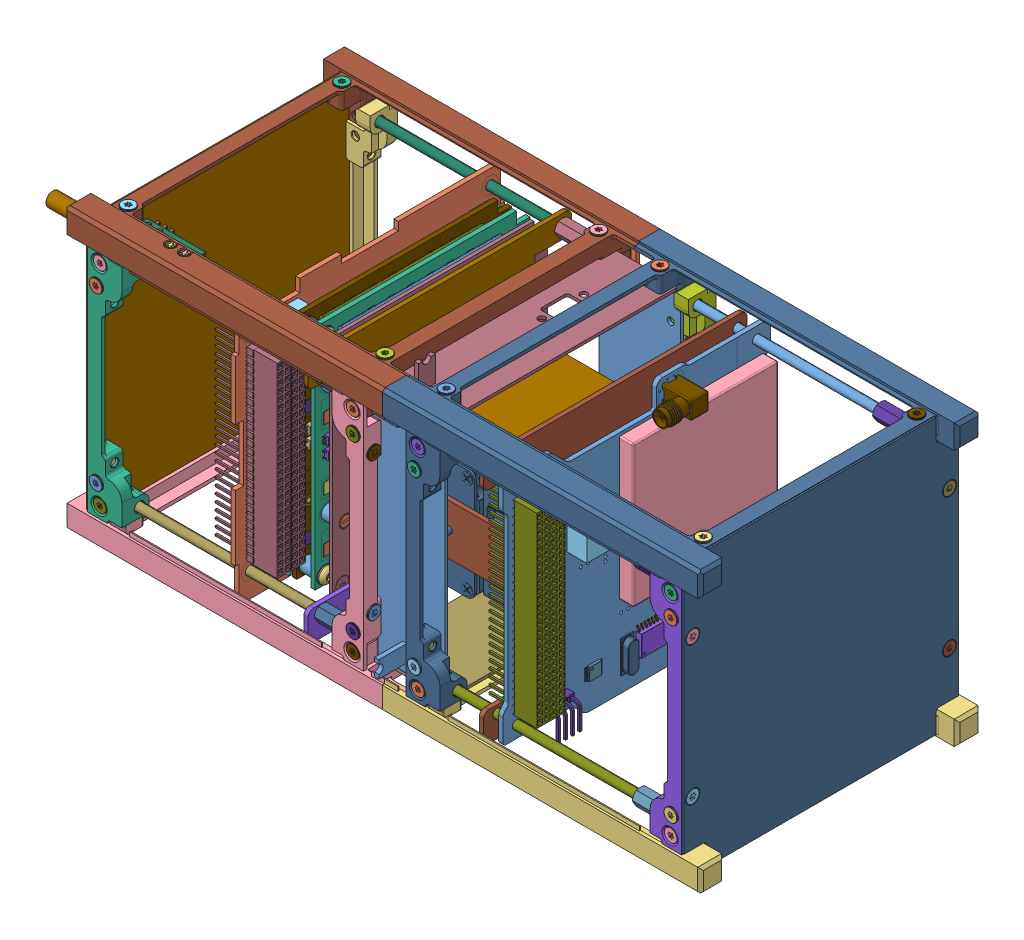
SolidWorks assembly V7A-YONSEI_ONLY_9JAN15, configuration Default. Lengths in mm. (continued)
Components (placement in the parent): (continued)
- EPS_ASM-1: EPS_ASM [Default] at (-345.0705 -361.6496 49.2336) x (0 1 0.000009) z (0 0.000009 -1) size (90.18 31.69 95.89) (continued)
  - ASM0003_ASM-1: ASM0003_ASM [Default] at origin size (90.18 31.69 95.89) (continued)
    - ASM0011_ASM-1: ASM0011_ASM [Default] at (362.3486 340.9078 -29.4212) size (84.27 11.35 76.64) (continued)
      - 3D-13-00246_ANY-2: 3D-13-00246_ANY [Default] at (54.4544 66.7437 67.4732) x (0 -1 0) z (0.000827 0 1) size (3.03 5.56 5.56)
      - R0603_ANY-13: R0603_ANY [Default] at (14.7573 68.2437 69.863) x (0 0 -1) z (-1 0 0) size (1.6 0.55 0.8)
      - R0603_ANY-14: R0603_ANY [Default] at (44.403 69.8437 66.9107) size (1.6 0.55 0.8)
      - SOT-23-5_ANY_ASM-2: SOT-23-5_ANY_ASM [Default] at (31.7757 70.5687 0.0073) size (3.05 1.45 3)
        - NONE-108284-1: NONE-108284 [Default] at origin size (0.4 0.83 0.63)
        - NONE-108285-1: NONE-108285 [Default] at origin size (3.05 1.45 1.75)
        - NONE-108289-1: NONE-108289 [Default] at origin size (0.4 0.83 0.63)
        - NONE-108292-1: NONE-108292 [Default] at origin size (0.4 0.83 0.63)
        - NONE-108294-1: NONE-108294 [Default] at origin size (0.4 0.83 0.63)
        - NONE-108296-1: NONE-108296 [Default] at origin size (0.4 0.83 0.63)
        - NONE-108297-1: NONE-108297 [Default] at origin size (0.4 0.83 0.63)
      - KX14-20K2DE_ANY-1: KX14-20K2DE_ANY [Default] at (31.8644 69.8937 66.8242) x (-1 0 0) z (0 0 -1) size (17.4 4.15 6.4)
      - R0603_ANY-15: R0603_ANY [Default] at (12.594 68.2437 69.8309) x (0 0 -1) z (-1 0 0) size (1.6 0.55 0.8)
      - 3_7V_BATTERY_ANY_ASM-2: 3_7V_BATTERY_ANY_ASM [Default] at (51.6059 69.8437 3.8964) x (0 0 1) z (-1 0 0) size (62.81 5 35.56)
        - NONE-26123-1: NONE-26123 [Default] at origin size (57.81 5 35.56)
        - NONE-26132-1: NONE-26132 [Default] at origin size (5 0.1 4)
        - NONE-26143-1: NONE-26143 [Default] at origin size (5 0.1 4)
      - R0603_ANY-16: R0603_ANY [Default] at (-9.55 69.8437 61.8847) size (1.6 0.55 0.8)
      - 3D-13-00246_ANY-3: 3D-13-00246_ANY [Default] at (53.4544 66.7437 0.4732) x (0 -1 0) z (-0.554303 0 0.832315) size (3.03 5.56 5.56)
      - R0603_ANY-17: R0603_ANY [Default] at (31.703 69.8437 38.3357) size (1.6 0.55 0.8)
      - R0603_ANY-18: R0603_ANY [Default] at (11.21 68.2437 62.1158) x (0 0 -1) z (-1 0 0) size (1.6 0.55 0.8)
      - C0603_ANY-2: C0603_ANY [Default] at (15.4552 68.2437 64.3707) x (0 0 -1) z (-1 0 0) size (1.6 0.9 0.8)
      - 3D-13-00246_ANY-4: 3D-13-00246_ANY [Default] at (13.4544 66.7437 0.4732) x (0 -1 0) z (0.000827 0 1) size (3.03 5.56 5.56)
      - TSSOP-8_AA__TSSOP-8__ANY-1: TSSOP-8_AA__TSSOP-8__ANY [Default] at (-9.5164 68.2437 62.3436) x (-0.000827 0 -1) z (-1 0 0.000827) size (6.46 1.2 3)
      - 3D-11-00227-REVA_ANY-1: 3D-11-00227-REVA_ANY [Default] at (-360.7506 69.8437 429.8122) x (1 0 0) z (0 1 0) size (84.27 76.64 1.72)
      - MINIMELF_DOMYSLNA_ANY-2: MINIMELF_DOMYSLNA_ANY [Default] at (41.9699 67.4437 0.9077) x (0 0 -1) z (-1 0 0) size (3.7 1.6 1.6)
      - SO-8_ANY-1: SO-8_ANY [Default] at (15.6729 70.8695 69.1672) x (0 0 -1) z (1 0 0) size (5.01 1.9 6.34)
      - R0603_ANY-19: R0603_ANY [Default] at (-9.1235 68.2437 56.9927) x (1 0 0) z (0 0 -1) size (1.6 0.55 0.8)
      - R0603_ANY-20: R0603_ANY [Default] at (17.6855 68.2437 64.387) x (0 0 -1) z (-1 0 0) size (1.6 0.55 0.8)
    - PRT0361-4: PRT0361 [Default] at (356.88 419.2115 -30.0115) x (0 -1 0) z (0.364885 0 0.931052) size (13.97 5.77 5.75)
    - PRT0359-6: PRT0359 [Default] at (416.803 422.3515 38.052) size (5.1 5.01 5.1)
    - PRT0359-7: PRT0359 [Default] at (369.803 422.3515 38.052) x (-0.201796 0 -0.979428) z (0.979428 0 -0.201796) size (5.1 5.01 5.1)
    - PRT0360-2: PRT0360 [Default] at (375.803 423.5515 -28.948) x (0 -1 0) z (0 0 1) size (10 3.8 3.77)
    - PRT0336-4: PRT0336 [Default] at (356.88 417.3615 -30.0115) x (0 -1 0) z (-0.82939 0 -0.55867) size (0.2 6 6)
    - PRT0360-3: PRT0360 [Default] at (369.803 423.5515 38.052) x (0 -1 0) z (0 0 1) size (10 3.8 3.77)
    - PRT0360-4: PRT0360 [Default] at (416.803 423.5515 38.052) x (0 -1 0) z (0 0 1) size (10 3.8 3.77)
    - PRT0359-8: PRT0359 [Default] at (375.803 422.3515 -28.948) x (0.95979 0 0.280718) z (-0.280718 0 0.95979) size (5.1 5.01 5.1)
- NANOCOM_ASM-1: NANOCOM_ASM [Default] at (152.6886 77.8142 2.1033) x (0 -0.000104 1) z (1 0 0) size (95.47 90.17 20.02)
  - ASM0012_ASM-1: ASM0012_ASM [Default] at origin size (95.47 90.17 20.02)
    - PRT0335-1: PRT0335 [Default] at origin size (95.47 90.17 1.6)
    - PRT0427-1: PRT0427 [Default] at (32.42 14.7398 4.9503) x (1 0.000012 0) z (-0.000012 1 0) size (8.12 3.8 9.75)
    - PRT0427-2: PRT0427 [Default] at (15.7996 44.1896 4.9503) x (-0.000012 1 0) z (-1 -0.000012 0) size (8.12 3.8 9.75)
    - PRT0427-3: PRT0427 [Default] at (52.7197 35.9501 4.9503) x (1 0.000012 0) z (-0.000012 1 0) size (8.12 3.8 9.75)
    - PRT0428-1: PRT0428 [Default] at (50.8249 50.0202 4.5503) x (-0.000012 1 0) z (0 0 -1) size (6.6 5.1 3.1)
    - PRT0429-1: PRT0429 [Default] at (50.369 28.293 1.5503) x (-0.000012 1 0) z (0 0 1) size (50.4 51.7 5)
    - PRT0430-1: PRT0430 [Default] at (59.7297 38.0301 1.55) x (1 0.000012 0) z (0 0 1) size (13 13 7)
    - PRT0431-1: PRT0431 [Default] at (67.2549 52.3904 -0.05) x (-0.000012 1 0) z (0 0 -1) size (6.6 5.1 3.1)
    - PRT0428-2: PRT0428 [Default] at (16.1742 49.6995 4.55) x (0.000012 -1 0) z (0 0 -1) size (6.6 5.1 3.1)
    - PRT0432-1: PRT0432 [Default] at (17.675 87.1 3.25) size (15.15 5.2 3.4)
    - ASM0013_ASM-1: ASM0013_ASM [Default] at (45.9517 54.2125 1.61) x (0.000012 -1 0) z (0 0 1) size (10.7 12.5 2.06)
      - PRT0433-1: PRT0433 [Default] at origin size (7.5 12.5 2)
      - PRT0434-1: PRT0434 [Default] at (-30.3036 -9.9322 -5.7208) x (-1 0 0) z (0 1 0) size (1.6 1 0.5)
      - PRT0434-2: PRT0434 [Default] at (-30.3036 -8.6622 -5.7208) x (-1 0 0) z (0 1 0) size (1.6 1 0.5)
      - PRT0434-3: PRT0434 [Default] at (-30.3036 -7.3922 -5.7208) x (-1 0 0) z (0 1 0) size (1.6 1 0.5)
      - PRT0434-4: PRT0434 [Default] at (-30.3036 -6.1222 -5.7208) x (-1 0 0) z (0 1 0) size (1.6 1 0.5)
      - PRT0434-5: PRT0434 [Default] at (-30.3036 -4.8522 -5.7208) x (-1 0 0) z (0 1 0) size (1.6 1 0.5)
      - PRT0434-6: PRT0434 [Default] at (-30.3036 -3.5822 -5.7208) x (-1 0 0) z (0 1 0) size (1.6 1 0.5)
      - PRT0434-7: PRT0434 [Default] at (-30.3036 -2.3122 -5.7208) x (-1 0 0) z (0 1 0) size (1.6 1 0.5)
      - PRT0434-8: PRT0434 [Default] at (-30.3036 -1.0422 -5.7208) x (-1 0 0) z (0 1 0) size (1.6 1 0.5)
      - PRT0434-9: PRT0434 [Default] at (-30.3036 0.2278 -5.7208) x (-1 0 0) z (0 1 0) size (1.6 1 0.5)
      - PRT0434-10: PRT0434 [Default] at (-30.3036 1.4978 -5.7208) x (-1 0 0) z (0 1 0) size (1.6 1 0.5)
      - PRT0434-11: PRT0434 [Default] at (-16.1712 1.9678 -5.7208) x (1 0 0) z (0 -1 0) size (1.6 1 0.5)
      - PRT0434-12: PRT0434 [Default] at (-16.1712 0.6978 -5.7208) x (1 0 0) z (0 -1 0) size (1.6 1 0.5)
      - PRT0434-13: PRT0434 [Default] at (-16.1712 -0.5722 -5.7208) x (1 0 0) z (0 -1 0) size (1.6 1 0.5)
      - PRT0434-14: PRT0434 [Default] at (-16.1712 -1.8422 -5.7208) x (1 0 0) z (0 -1 0) size (1.6 1 0.5)
      - PRT0434-15: PRT0434 [Default] at (-16.1712 -3.1122 -5.7208) x (1 0 0) z (0 -1 0) size (1.6 1 0.5)
      - PRT0434-16: PRT0434 [Default] at (-16.1712 -4.3822 -5.7208) x (1 0 0) z (0 -1 0) size (1.6 1 0.5)
      - PRT0434-17: PRT0434 [Default] at (-16.1712 -5.6522 -5.7208) x (1 0 0) z (0 -1 0) size (1.6 1 0.5)
      - PRT0434-18: PRT0434 [Default] at (-16.1712 -6.9222 -5.7208) x (1 0 0) z (0 -1 0) size (1.6 1 0.5)
      - PRT0434-19: PRT0434 [Default] at (-16.1712 -8.1922 -5.7208) x (1 0 0) z (0 -1 0) size (1.6 1 0.5)
      - PRT0434-20: PRT0434 [Default] at (-16.1712 -9.4622 -5.7208) x (1 0 0) z (0 -1 0) size (1.6 1 0.5)
    - PRT0435-1: PRT0435 [Default] at (52.9769 89.7275 1.55) x (-0.000012 1 0) z (0 0 1) size (11.4 4.5 2.6)
    - PRT0436-1: PRT0436 [Default] at (10.9667 64.722 1.55) x (-0.000012 1 0) z (0 0 1) size (3.4 1.7 1.3)
    - ASM0150_ASM-1: ASM0150_ASM [Default] at (48.2268 68.5178 -0.06) x (1 0.000012 0) z (0 0 -1) size (21.91 21.91 0.92)
      - PRT0437-1: PRT0437 [Default] at origin size (20 20 0.86)
      - PRT0438-1: PRT0438 [Default] at (-25.9374 -6.5504 -5.8759) x (0 1 0) z (1 0 0) size (0.95 0.58 0.3)
      - PRT0438-2: PRT0438 [Default] at (-25.4374 -6.5504 -5.8759) x (0 1 0) z (1 0 0) size (0.95 0.58 0.3)
      - PRT0438-3: PRT0438 [Default] at (-24.9374 -6.5504 -5.8759) x (0 1 0) z (1 0 0) size (0.95 0.58 0.3)
      - PRT0438-4: PRT0438 [Default] at (-24.4374 -6.5504 -5.8759) x (0 1 0) z (1 0 0) size (0.95 0.58 0.3)
      - PRT0438-5: PRT0438 [Default] at (-23.9374 -6.5504 -5.8759) x (0 1 0) z (1 0 0) size (0.95 0.58 0.3)
      - PRT0438-6: PRT0438 [Default] at (-23.4374 -6.5504 -5.8759) x (0 1 0) z (1 0 0) size (0.95 0.58 0.3)
      - PRT0438-7: PRT0438 [Default] at (-22.9374 -6.5504 -5.8759) x (0 1 0) z (1 0 0) size (0.95 0.58 0.3)
      - PRT0438-8: PRT0438 [Default] at (-22.4374 -6.5504 -5.8759) x (0 1 0) z (1 0 0) size (0.95 0.58 0.3)
      - PRT0438-9: PRT0438 [Default] at (-21.9374 -6.5504 -5.8759) x (0 1 0) z (1 0 0) size (0.95 0.58 0.3)
      - PRT0438-10: PRT0438 [Default] at (-21.4374 -6.5504 -5.8759) x (0 1 0) z (1 0 0) size (0.95 0.58 0.3)
      - PRT0438-11: PRT0438 [Default] at (-20.9374 -6.5504 -5.8759) x (0 1 0) z (1 0 0) size (0.95 0.58 0.3)
      - PRT0438-12: PRT0438 [Default] at (-20.4374 -6.5504 -5.8759) x (0 1 0) z (1 0 0) size (0.95 0.58 0.3)
      - PRT0438-13: PRT0438 [Default] at (-19.9374 -6.5504 -5.8759) x (0 1 0) z (1 0 0) size (0.95 0.58 0.3)
      - PRT0438-14: PRT0438 [Default] at (-19.4374 -6.5504 -5.8759) x (0 1 0) z (1 0 0) size (0.95 0.58 0.3)
      - PRT0438-15: PRT0438 [Default] at (-18.9374 -6.5504 -5.8759) x (0 1 0) z (1 0 0) size (0.95 0.58 0.3)
      - PRT0438-16: PRT0438 [Default] at (-18.4374 -6.5504 -5.8759) x (0 1 0) z (1 0 0) size (0.95 0.58 0.3)
      - PRT0438-17: PRT0438 [Default] at (-17.9374 -6.5504 -5.8759) x (0 1 0) z (1 0 0) size (0.95 0.58 0.3)
      - PRT0438-18: PRT0438 [Default] at (-17.4374 -6.5504 -5.8759) x (0 1 0) z (1 0 0) size (0.95 0.58 0.3)
      - PRT0438-19: PRT0438 [Default] at (-16.9374 -6.5504 -5.8759) x (0 1 0) z (1 0 0) size (0.95 0.58 0.3)
      - PRT0438-20: PRT0438 [Default] at (-16.4374 -6.5504 -5.8759) x (0 1 0) z (1 0 0) size (0.95 0.58 0.3)
      - PRT0438-21: PRT0438 [Default] at (-15.9374 -6.5504 -5.8759) x (0 1 0) z (1 0 0) size (0.95 0.58 0.3)
      - PRT0438-22: PRT0438 [Default] at (-15.4374 -6.5504 -5.8759) x (0 1 0) z (1 0 0) size (0.95 0.58 0.3)
      - PRT0438-23: PRT0438 [Default] at (-14.9374 -6.5504 -5.8759) x (0 1 0) z (1 0 0) size (0.95 0.58 0.3)
      - PRT0438-24: PRT0438 [Default] at (-14.4374 -6.5504 -5.8759) x (0 1 0) z (1 0 0) size (0.95 0.58 0.3)
      - PRT0438-25: PRT0438 [Default] at (-13.9374 -6.5504 -5.8759) x (0 1 0) z (1 0 0) size (0.95 0.58 0.3)
      - PRT0438-26: PRT0438 [Default] at (-13.4374 -6.5504 -5.8759) x (0 1 0) z (1 0 0) size (0.95 0.58 0.3)
      - PRT0438-27: PRT0438 [Default] at (-12.9374 -6.5504 -5.8759) x (0 1 0) z (1 0 0) size (0.95 0.58 0.3)
      - PRT0438-28: PRT0438 [Default] at (-12.4374 -6.5504 -5.8759) x (0 1 0) z (1 0 0) size (0.95 0.58 0.3)
      - PRT0438-29: PRT0438 [Default] at (-11.9374 -6.5504 -5.8759) x (0 1 0) z (1 0 0) size (0.95 0.58 0.3)
      - PRT0438-30: PRT0438 [Default] at (-11.4374 -6.5504 -5.8759) x (0 1 0) z (1 0 0) size (0.95 0.58 0.3)
      - PRT0438-31: PRT0438 [Default] at (-10.9374 -6.5504 -5.8759) x (0 1 0) z (1 0 0) size (0.95 0.58 0.3)
      - PRT0438-32: PRT0438 [Default] at (-10.4374 -6.5504 -5.8759) x (0 1 0) z (1 0 0) size (0.95 0.58 0.3)
      - PRT0438-33: PRT0438 [Default] at (-9.9374 -6.5504 -5.8759) x (0 1 0) z (1 0 0) size (0.95 0.58 0.3)
      - PRT0438-34: PRT0438 [Default] at (-9.4374 -6.5504 -5.8759) x (0 1 0) z (1 0 0) size (0.95 0.58 0.3)
      - PRT0438-35: PRT0438 [Default] at (-8.9374 -6.5504 -5.8759) x (0 1 0) z (1 0 0) size (0.95 0.58 0.3)
      - PRT0438-36: PRT0438 [Default] at (-8.4374 -6.5504 -5.8759) x (0 1 0) z (1 0 0) size (0.95 0.58 0.3)
      - PRT0438-37: PRT0438 [Default] at (-25.6374 -8.914 -5.8759) x (0 -1 0) z (-1 0 0) size (0.95 0.58 0.3)
      - PRT0438-38: PRT0438 [Default] at (-25.1374 -8.914 -5.8759) x (0 -1 0) z (-1 0 0) size (0.95 0.58 0.3)
      - PRT0438-39: PRT0438 [Default] at (-24.6374 -8.914 -5.8759) x (0 -1 0) z (-1 0 0) size (0.95 0.58 0.3)
      - PRT0438-40: PRT0438 [Default] at (-24.1374 -8.914 -5.8759) x (0 -1 0) z (-1 0 0) size (0.95 0.58 0.3)
      - PRT0438-41: PRT0438 [Default] at (-23.6374 -8.914 -5.8759) x (0 -1 0) z (-1 0 0) size (0.95 0.58 0.3)
      - PRT0438-42: PRT0438 [Default] at (-23.1374 -8.914 -5.8759) x (0 -1 0) z (-1 0 0) size (0.95 0.58 0.3)
      - PRT0438-43: PRT0438 [Default] at (-22.6374 -8.914 -5.8759) x (0 -1 0) z (-1 0 0) size (0.95 0.58 0.3)
      - PRT0438-44: PRT0438 [Default] at (-22.1374 -8.914 -5.8759) x (0 -1 0) z (-1 0 0) size (0.95 0.58 0.3)
      - PRT0438-45: PRT0438 [Default] at (-21.6374 -8.914 -5.8759) x (0 -1 0) z (-1 0 0) size (0.95 0.58 0.3)
      - PRT0438-46: PRT0438 [Default] at (-21.1374 -8.914 -5.8759) x (0 -1 0) z (-1 0 0) size (0.95 0.58 0.3)
      - PRT0438-47: PRT0438 [Default] at (-20.6374 -8.914 -5.8759) x (0 -1 0) z (-1 0 0) size (0.95 0.58 0.3)
      - PRT0438-48: PRT0438 [Default] at (-20.1374 -8.914 -5.8759) x (0 -1 0) z (-1 0 0) size (0.95 0.58 0.3)
      - PRT0438-49: PRT0438 [Default] at (-19.6374 -8.914 -5.8759) x (0 -1 0) z (-1 0 0) size (0.95 0.58 0.3)
      - PRT0438-50: PRT0438 [Default] at (-19.1374 -8.914 -5.8759) x (0 -1 0) z (-1 0 0) size (0.95 0.58 0.3)
      - PRT0438-51: PRT0438 [Default] at (-18.6374 -8.914 -5.8759) x (0 -1 0) z (-1 0 0) size (0.95 0.58 0.3)
      - PRT0438-52: PRT0438 [Default] at (-18.1374 -8.914 -5.8759) x (0 -1 0) z (-1 0 0) size (0.95 0.58 0.3)
      - PRT0438-53: PRT0438 [Default] at (-17.6374 -8.914 -5.8759) x (0 -1 0) z (-1 0 0) size (0.95 0.58 0.3)
      - PRT0438-54: PRT0438 [Default] at (-17.1374 -8.914 -5.8759) x (0 -1 0) z (-1 0 0) size (0.95 0.58 0.3)
      - PRT0438-55: PRT0438 [Default] at (-16.6374 -8.914 -5.8759) x (0 -1 0) z (-1 0 0) size (0.95 0.58 0.3)
      - PRT0438-56: PRT0438 [Default] at (-16.1374 -8.914 -5.8759) x (0 -1 0) z (-1 0 0) size (0.95 0.58 0.3)
      - PRT0438-57: PRT0438 [Default] at (-15.6374 -8.914 -5.8759) x (0 -1 0) z (-1 0 0) size (0.95 0.58 0.3)
      - PRT0438-58: PRT0438 [Default] at (-15.1374 -8.914 -5.8759) x (0 -1 0) z (-1 0 0) size (0.95 0.58 0.3)
      - PRT0438-59: PRT0438 [Default] at (-14.6374 -8.914 -5.8759) x (0 -1 0) z (-1 0 0) size (0.95 0.58 0.3)
      - PRT0438-60: PRT0438 [Default] at (-14.1374 -8.914 -5.8759) x (0 -1 0) z (-1 0 0) size (0.95 0.58 0.3)
      - PRT0438-61: PRT0438 [Default] at (-13.6374 -8.914 -5.8759) x (0 -1 0) z (-1 0 0) size (0.95 0.58 0.3)
      - PRT0438-62: PRT0438 [Default] at (-13.1374 -8.914 -5.8759) x (0 -1 0) z (-1 0 0) size (0.95 0.58 0.3)
      - PRT0438-63: PRT0438 [Default] at (-12.6374 -8.914 -5.8759) x (0 -1 0) z (-1 0 0) size (0.95 0.58 0.3)
      - PRT0438-64: PRT0438 [Default] at (-12.1374 -8.914 -5.8759) x (0 -1 0) z (-1 0 0) size (0.95 0.58 0.3)
      - PRT0438-65: PRT0438 [Default] at (-11.6374 -8.914 -5.8759) x (0 -1 0) z (-1 0 0) size (0.95 0.58 0.3)
      - PRT0438-66: PRT0438 [Default] at (-11.1374 -8.914 -5.8759) x (0 -1 0) z (-1 0 0) size (0.95 0.58 0.3)
      - PRT0438-67: PRT0438 [Default] at (-10.6374 -8.914 -5.8759) x (0 -1 0) z (-1 0 0) size (0.95 0.58 0.3)
      - PRT0438-68: PRT0438 [Default] at (-10.1374 -8.914 -5.8759) x (0 -1 0) z (-1 0 0) size (0.95 0.58 0.3)
      - PRT0438-69: PRT0438 [Default] at (-9.6374 -8.914 -5.8759) x (0 -1 0) z (-1 0 0) size (0.95 0.58 0.3)
      - PRT0438-70: PRT0438 [Default] at (-9.1374 -8.914 -5.8759) x (0 -1 0) z (-1 0 0) size (0.95 0.58 0.3)
      - PRT0438-71: PRT0438 [Default] at (-8.6374 -8.914 -5.8759) x (0 -1 0) z (-1 0 0) size (0.95 0.58 0.3)
      - PRT0438-72: PRT0438 [Default] at (-8.1374 -8.914 -5.8759) x (0 -1 0) z (-1 0 0) size (0.95 0.58 0.3)
      - PRT0438-73: PRT0438 [Default] at (-15.8057 1.2178 -5.8759) x (1 0 0) z (0 -1 0) size (0.95 0.58 0.3)
      - PRT0438-74: PRT0438 [Default] at (-15.8057 0.7178 -5.8759) x (1 0 0) z (0 -1 0) size (0.95 0.58 0.3)
      - PRT0438-75: PRT0438 [Default] at (-15.8057 0.2178 -5.8759) x (1 0 0) z (0 -1 0) size (0.95 0.58 0.3)
      - PRT0438-76: PRT0438 [Default] at (-15.8057 -0.2822 -5.8759) x (1 0 0) z (0 -1 0) size (0.95 0.58 0.3)
      - PRT0438-77: PRT0438 [Default] at (-15.8057 -0.7822 -5.8759) x (1 0 0) z (0 -1 0) size (0.95 0.58 0.3)
      - PRT0438-78: PRT0438 [Default] at (-15.8057 -1.2822 -5.8759) x (1 0 0) z (0 -1 0) size (0.95 0.58 0.3)
      - PRT0438-79: PRT0438 [Default] at (-15.8057 -1.7822 -5.8759) x (1 0 0) z (0 -1 0) size (0.95 0.58 0.3)
      - PRT0438-80: PRT0438 [Default] at (-15.8057 -2.2822 -5.8759) x (1 0 0) z (0 -1 0) size (0.95 0.58 0.3)
      - PRT0438-81: PRT0438 [Default] at (-15.8057 -2.7822 -5.8759) x (1 0 0) z (0 -1 0) size (0.95 0.58 0.3)
      - PRT0438-82: PRT0438 [Default] at (-15.8057 -3.2822 -5.8759) x (1 0 0) z (0 -1 0) size (0.95 0.58 0.3)
      - PRT0438-83: PRT0438 [Default] at (-15.8057 -3.7822 -5.8759) x (1 0 0) z (0 -1 0) size (0.95 0.58 0.3)
      - PRT0438-84: PRT0438 [Default] at (-15.8057 -4.2822 -5.8759) x (1 0 0) z (0 -1 0) size (0.95 0.58 0.3)
      - PRT0438-85: PRT0438 [Default] at (-15.8057 -4.7822 -5.8759) x (1 0 0) z (0 -1 0) size (0.95 0.58 0.3)
      - PRT0438-86: PRT0438 [Default] at (-15.8057 -5.2822 -5.8759) x (1 0 0) z (0 -1 0) size (0.95 0.58 0.3)
      - PRT0438-87: PRT0438 [Default] at (-15.8057 -5.7822 -5.8759) x (1 0 0) z (0 -1 0) size (0.95 0.58 0.3)
      - PRT0438-88: PRT0438 [Default] at (-15.8057 -6.2822 -5.8759) x (1 0 0) z (0 -1 0) size (0.95 0.58 0.3)
      - PRT0438-89: PRT0438 [Default] at (-15.8057 -6.7822 -5.8759) x (1 0 0) z (0 -1 0) size (0.95 0.58 0.3)
      - PRT0438-90: PRT0438 [Default] at (-15.8057 -7.2822 -5.8759) x (1 0 0) z (0 -1 0) size (0.95 0.58 0.3)
      - PRT0438-91: PRT0438 [Default] at (-15.8057 -7.7822 -5.8759) x (1 0 0) z (0 -1 0) size (0.95 0.58 0.3)
      - PRT0438-92: PRT0438 [Default] at (-15.8057 -8.2822 -5.8759) x (1 0 0) z (0 -1 0) size (0.95 0.58 0.3)
      - PRT0438-93: PRT0438 [Default] at (-15.8057 -8.7822 -5.8759) x (1 0 0) z (0 -1 0) size (0.95 0.58 0.3)
      - PRT0438-94: PRT0438 [Default] at (-15.8057 -9.2822 -5.8759) x (1 0 0) z (0 -1 0) size (0.95 0.58 0.3)
      - PRT0438-95: PRT0438 [Default] at (-15.8057 -9.7822 -5.8759) x (1 0 0) z (0 -1 0) size (0.95 0.58 0.3)
      - PRT0438-96: PRT0438 [Default] at (-15.8057 -10.2822 -5.8759) x (1 0 0) z (0 -1 0) size (0.95 0.58 0.3)
      - PRT0438-97: PRT0438 [Default] at (-15.8057 -10.7822 -5.8759) x (1 0 0) z (0 -1 0) size (0.95 0.58 0.3)
      - PRT0438-98: PRT0438 [Default] at (-15.8057 -11.2822 -5.8759) x (1 0 0) z (0 -1 0) size (0.95 0.58 0.3)
      - PRT0438-99: PRT0438 [Default] at (-15.8057 -11.7822 -5.8759) x (1 0 0) z (0 -1 0) size (0.95 0.58 0.3)
      - PRT0438-100: PRT0438 [Default] at (-15.8057 -12.2822 -5.8759) x (1 0 0) z (0 -1 0) size (0.95 0.58 0.3)
      - PRT0438-101: PRT0438 [Default] at (-15.8057 -12.7822 -5.8759) x (1 0 0) z (0 -1 0) size (0.95 0.58 0.3)
      - PRT0438-102: PRT0438 [Default] at (-15.8057 -13.2822 -5.8759) x (1 0 0) z (0 -1 0) size (0.95 0.58 0.3)
      - PRT0438-103: PRT0438 [Default] at (-15.8057 -13.7822 -5.8759) x (1 0 0) z (0 -1 0) size (0.95 0.58 0.3)
      - PRT0438-104: PRT0438 [Default] at (-15.8057 -14.2822 -5.8759) x (1 0 0) z (0 -1 0) size (0.95 0.58 0.3)
      - PRT0438-105: PRT0438 [Default] at (-15.8057 -14.7822 -5.8759) x (1 0 0) z (0 -1 0) size (0.95 0.58 0.3)
      - PRT0438-106: PRT0438 [Default] at (-15.8057 -15.2822 -5.8759) x (1 0 0) z (0 -1 0) size (0.95 0.58 0.3)
      - PRT0438-107: PRT0438 [Default] at (-15.8057 -15.7822 -5.8759) x (1 0 0) z (0 -1 0) size (0.95 0.58 0.3)
      - PRT0438-108: PRT0438 [Default] at (-15.8057 -16.2822 -5.8759) x (1 0 0) z (0 -1 0) size (0.95 0.58 0.3)
      - PRT0438-109: PRT0438 [Default] at (-18.1692 -16.6422 -5.7559) x (-1 0 0) z (0 1 0) size (0.95 0.58 0.3)
      - PRT0438-110: PRT0438 [Default] at (-18.1692 -16.1422 -5.7559) x (-1 0 0) z (0 1 0) size (0.95 0.58 0.3)
      - PRT0438-111: PRT0438 [Default] at (-18.1692 -15.6422 -5.7559) x (-1 0 0) z (0 1 0) size (0.95 0.58 0.3)
      - PRT0438-112: PRT0438 [Default] at (-18.1692 -15.1422 -5.7559) x (-1 0 0) z (0 1 0) size (0.95 0.58 0.3)
      - PRT0438-113: PRT0438 [Default] at (-18.1692 -14.6422 -5.7559) x (-1 0 0) z (0 1 0) size (0.95 0.58 0.3)
      - PRT0438-114: PRT0438 [Default] at (-18.1692 -14.1422 -5.7559) x (-1 0 0) z (0 1 0) size (0.95 0.58 0.3)
      - PRT0438-115: PRT0438 [Default] at (-18.1692 -13.6422 -5.7559) x (-1 0 0) z (0 1 0) size (0.95 0.58 0.3)
      - PRT0438-116: PRT0438 [Default] at (-18.1692 -13.1422 -5.7559) x (-1 0 0) z (0 1 0) size (0.95 0.58 0.3)
      - PRT0438-117: PRT0438 [Default] at (-18.1692 -12.6422 -5.7559) x (-1 0 0) z (0 1 0) size (0.95 0.58 0.3)
      - PRT0438-118: PRT0438 [Default] at (-18.1692 -12.1422 -5.7559) x (-1 0 0) z (0 1 0) size (0.95 0.58 0.3)
      - PRT0438-119: PRT0438 [Default] at (-18.1692 -11.6422 -5.7559) x (-1 0 0) z (0 1 0) size (0.95 0.58 0.3)
      - PRT0438-120: PRT0438 [Default] at (-18.1692 -11.1422 -5.7559) x (-1 0 0) z (0 1 0) size (0.95 0.58 0.3)
      - PRT0438-121: PRT0438 [Default] at (-18.1692 -10.6422 -5.7559) x (-1 0 0) z (0 1 0) size (0.95 0.58 0.3)
      - PRT0438-122: PRT0438 [Default] at (-18.1692 -10.1422 -5.7559) x (-1 0 0) z (0 1 0) size (0.95 0.58 0.3)
      - PRT0438-123: PRT0438 [Default] at (-18.1692 -9.6422 -5.7559) x (-1 0 0) z (0 1 0) size (0.95 0.58 0.3)
      - PRT0438-124: PRT0438 [Default] at (-18.1692 -9.1422 -5.7559) x (-1 0 0) z (0 1 0) size (0.95 0.58 0.3)
      - PRT0438-125: PRT0438 [Default] at (-18.1692 -8.6422 -5.7559) x (-1 0 0) z (0 1 0) size (0.95 0.58 0.3)
      - PRT0438-126: PRT0438 [Default] at (-18.1692 -8.1422 -5.7559) x (-1 0 0) z (0 1 0) size (0.95 0.58 0.3)
      - PRT0438-127: PRT0438 [Default] at (-18.1692 -7.6422 -5.7559) x (-1 0 0) z (0 1 0) size (0.95 0.58 0.3)
      - PRT0438-128: PRT0438 [Default] at (-18.1692 -7.1422 -5.7559) x (-1 0 0) z (0 1 0) size (0.95 0.58 0.3)
      - PRT0438-129: PRT0438 [Default] at (-18.1692 -6.6422 -5.7559) x (-1 0 0) z (0 1 0) size (0.95 0.58 0.3)
      - PRT0438-130: PRT0438 [Default] at (-18.1692 -6.1422 -5.7559) x (-1 0 0) z (0 1 0) size (0.95 0.58 0.3)
      - PRT0438-131: PRT0438 [Default] at (-18.1692 -5.6422 -5.7559) x (-1 0 0) z (0 1 0) size (0.95 0.58 0.3)
      - PRT0438-132: PRT0438 [Default] at (-18.1692 -5.1422 -5.7559) x (-1 0 0) z (0 1 0) size (0.95 0.58 0.3)
      - PRT0438-133: PRT0438 [Default] at (-18.1692 -4.6422 -5.7559) x (-1 0 0) z (0 1 0) size (0.95 0.58 0.3)
      - PRT0438-134: PRT0438 [Default] at (-18.1692 -4.1422 -5.7559) x (-1 0 0) z (0 1 0) size (0.95 0.58 0.3)
      - PRT0438-135: PRT0438 [Default] at (-18.1692 -3.6422 -5.7559) x (-1 0 0) z (0 1 0) size (0.95 0.58 0.3)
      - PRT0438-136: PRT0438 [Default] at (-18.1692 -3.1422 -5.7559) x (-1 0 0) z (0 1 0) size (0.95 0.58 0.3)
      - PRT0438-137: PRT0438 [Default] at (-18.1692 -2.6422 -5.7559) x (-1 0 0) z (0 1 0) size (0.95 0.58 0.3)
      - PRT0438-138: PRT0438 [Default] at (-18.1692 -2.1422 -5.7559) x (-1 0 0) z (0 1 0) size (0.95 0.58 0.3)
      - PRT0438-139: PRT0438 [Default] at (-18.1692 -1.6422 -5.7559) x (-1 0 0) z (0 1 0) size (0.95 0.58 0.3)
      - PRT0438-140: PRT0438 [Default] at (-18.1692 -1.1422 -5.7559) x (-1 0 0) z (0 1 0) size (0.95 0.58 0.3)
      - PRT0438-141: PRT0438 [Default] at (-18.1692 -0.6422 -5.7559) x (-1 0 0) z (0 1 0) size (0.95 0.58 0.3)
      - PRT0438-142: PRT0438 [Default] at (-18.1692 -0.1422 -5.7559) x (-1 0 0) z (0 1 0) size (0.95 0.58 0.3)
      - PRT0438-143: PRT0438 [Default] at (-18.1692 0.3578 -5.7559) x (-1 0 0) z (0 1 0) size (0.95 0.58 0.3)
      - PRT0438-144: PRT0438 [Default] at (-18.1692 0.8578 -5.7559) x (-1 0 0) z (0 1 0) size (0.95 0.58 0.3)
    - ASM0151_ASM-1: ASM0151_ASM [Default] at (38.7018 78.0677 1.61) x (-1 -0.000012 0) z (0 0 1) size (6.31 4.5 0.92)
      - PRT0439-1: PRT0439 [Default] at origin size (4.4 4.5 0.86)
      - LM70-PIN-1: LM70-PIN [Default] at (-33.7692 -2.0822 -5.8759) x (-1 0 0) z (0 1 0) size (0.95 0.58 0.3)
      - LM70-PIN-2: LM70-PIN [Default] at (-33.7692 -1.4322 -5.8759) x (-1 0 0) z (0 1 0) size (0.95 0.58 0.3)
      - LM70-PIN-3: LM70-PIN [Default] at (-33.7692 -0.7822 -5.8759) x (-1 0 0) z (0 1 0) size (0.95 0.58 0.3)
      - LM70-PIN-4: LM70-PIN [Default] at (-33.7692 -0.1322 -5.8759) x (-1 0 0) z (0 1 0) size (0.95 0.58 0.3)
      - LM70-PIN-5: LM70-PIN [Default] at (-33.7692 0.5178 -5.8759) x (-1 0 0) z (0 1 0) size (0.95 0.58 0.3)
      - LM70-PIN-6: LM70-PIN [Default] at (-33.7692 1.1678 -5.8759) x (-1 0 0) z (0 1 0) size (0.95 0.58 0.3)
      - LM70-PIN-7: LM70-PIN [Default] at (-33.7692 1.8178 -5.8759) x (-1 0 0) z (0 1 0) size (0.95 0.58 0.3)
      - LM70-PIN-8: LM70-PIN [Default] at (-15.8057 2.1178 -5.8759) x (1 0 0) z (0 -1 0) size (0.95 0.58 0.3)
      - LM70-PIN-9: LM70-PIN [Default] at (-15.8057 1.4678 -5.8759) x (1 0 0) z (0 -1 0) size (0.95 0.58 0.3)
      - LM70-PIN-10: LM70-PIN [Default] at (-15.8057 0.8178 -5.8759) x (1 0 0) z (0 -1 0) size (0.95 0.58 0.3)
      - LM70-PIN-11: LM70-PIN [Default] at (-15.8057 0.1678 -5.8759) x (1 0 0) z (0 -1 0) size (0.95 0.58 0.3)
      - LM70-PIN-12: LM70-PIN [Default] at (-15.8057 -0.4822 -5.8759) x (1 0 0) z (0 -1 0) size (0.95 0.58 0.3)
      - LM70-PIN-13: LM70-PIN [Default] at (-15.8057 -1.1322 -5.8759) x (1 0 0) z (0 -1 0) size (0.95 0.58 0.3)
      - LM70-PIN-14: LM70-PIN [Default] at (-15.8057 -1.7822 -5.8759) x (1 0 0) z (0 -1 0) size (0.95 0.58 0.3)
    - PRT0440-1: PRT0440 [Default] at (104.9379 60.2312 10.05) x (1 0 0) z (0 0 -1) size (10 66.5 18)
    - PRT0441-1: PRT0441 [Default] at (78 79.973 3.201) x (-1 0 0) z (0 1 0) size (9.91 9.45 10.08)
    - PRT0442-1: PRT0442 [Default] at (46.8 5.2711 8.8003) x (-0.001909 0.999998 0) z (0.999998 0.001909 0) size (6.36 13.94 14.21)
- GOMX-INTERSTAGE-B-1: GOMX-INTERSTAGE-B [Default] at (98.95 -7.925 8.1) x (0 1 0) z (0 0 -1) size (82.5 29 11)
- GOMX-INTERSTAGE-B-2: GOMX-INTERSTAGE-B [Default] at (98.95 74.575 91.2) x (0 -1 0) z (0 0 1) size (82.5 29 11)
